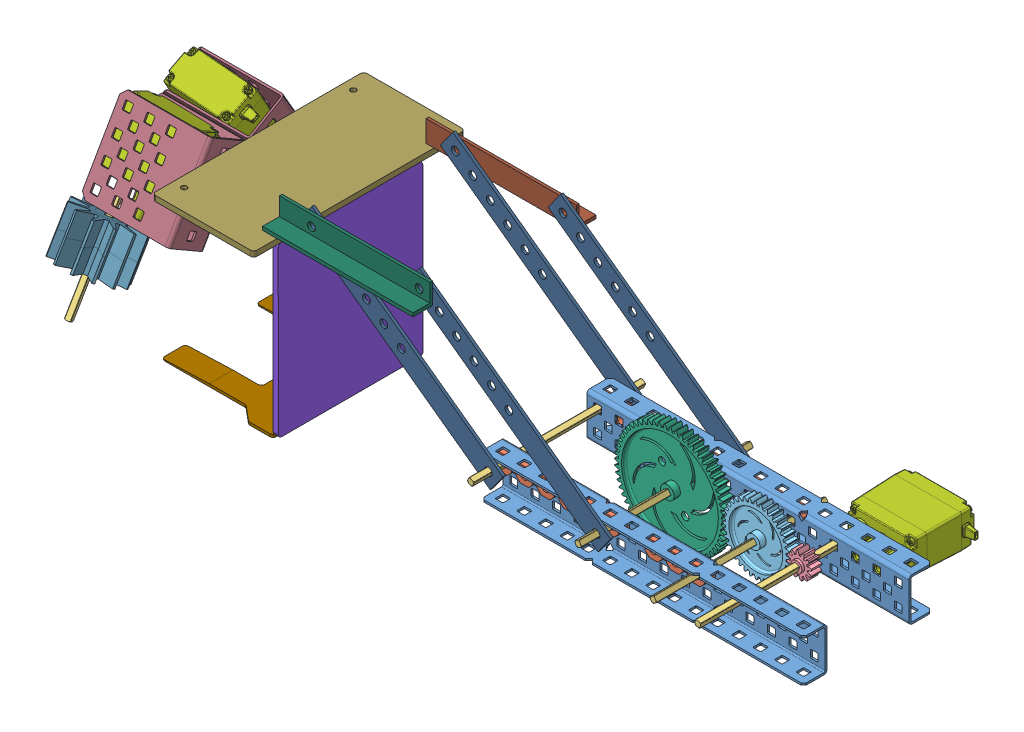
SolidWorks assembly LiftAssy-NoMates, configuration Default. Lengths in mm.
Overall size (436.18 185.84 157.73).
36 component instances, 15 part files, 3 mates.
Components (placement in the parent):
- VL-CHAN-121-15 RevA-1: VL-CHAN-121-15 RevA [Default] at (-291.0348 35.1994 12.7) x (1 0 0) z (0 -1 0) size (190.5 13.87 25.4)
- VL-CHAN-121-15 RevA-2: VL-CHAN-121-15 RevA [Default] at (-153.4652 35.1994 63.5) x (-1 0 0) z (0 -1 0) size (190.5 13.87 25.4)
- BEARING-FLAT-1: BEARING-FLAT [Default] at (-272.0848 31.6992 -76.2762) x (0 0 1) z (0 -1 0) size (7.04 35.56 10.16)
- BEARING-FLAT-2: BEARING-FLAT [Default] at (-233.9848 31.8008 -76.2762) x (0 0 1) z (0 -1 0) size (7.04 35.56 10.16)
- BEARING-FLAT-3: BEARING-FLAT [Default] at (-183.1848 57.2008 152.4762) x (0 0 -1) z (0 1 0) size (7.04 35.56 10.16)
- BEARING-FLAT-4: BEARING-FLAT [Default] at (-235.9152 57.2008 -76.2762) x (0 0 1) z (0 1 0) size (7.04 35.56 10.16)
- BEARING-FLAT-5: BEARING-FLAT [Default] at (-233.9848 57.2008 152.4762) x (0 0 -1) z (0 1 0) size (7.04 35.56 10.16)
- BEARING-FLAT-6: BEARING-FLAT [Default] at (-272.0848 57.2008 152.4762) x (0 0 -1) z (0 1 0) size (7.04 35.56 10.16)
- SHAFT-4000-1: SHAFT-4000 [Default] at (-311.2008 44.5008 38.1) x (0.41269 0.910872 0) z (0 0 1) size (4.18 4.18 101.81)
- SHAFT-4000-2: SHAFT-4000 [Default] at (-247.7008 44.5008 38.1) x (0.537594 -0.843204 0) z (0 0 1) size (4.18 4.18 101.81)
- SHAFT-4000-3: SHAFT-4000 [Default] at (-196.9008 44.5008 44.45) x (0.810991 0.585059 0) z (0 0 1) size (4.18 4.18 101.81)
- SHAFT-4000-4: SHAFT-4000 [Default] at (-171.4187 44.4677 43.6) x (0.963526 -0.267616 0) z (0 0 1) size (4.18 4.18 101.81)
- VEX-12-TOOTH-GEAR-1: VEX-12-TOOTH-GEAR [Default] at (-171.388 44.4851 31.3309) x (0.963526 -0.267616 0) z (0 0 1) size (14.8 14.8 9.53)
- VEX-36-TOOTH-GEAR-1: VEX-36-TOOTH-GEAR [Default] at (-196.9357 44.5064 31.3309) x (0.810991 0.585059 0) z (0 0 1) size (40.08 40.08 9.53)
- VEX-60-TOOTH-GEAR-1: VEX-60-TOOTH-GEAR [Default] at (-247.7353 44.5084 31.3309) x (0.537594 -0.843204 0) z (0 0 1) size (65.54 65.54 9.53)
- VEX-2WIRE-MOTOR-1: VEX-2WIRE-MOTOR [Default] at (-160.3202 44.45 -30.5) x (-1 0 0) z (0 0 -1) size (46.4 20 51.81)
- Pyramid Intake-1: Pyramid Intake [Default] at (-389.3852 43.5371 -4.7167) x (0 0 1) z (-0.989362 0.145478 0) size (150.3 140.72 320.47)
  - back-1: back [Default] at (51.2746 60.4405 44.4758) x (1 0 0) z (0 -0.146963 0.989142) size (85.5 99.5 3.17)
  - BottomForklift-1: BottomForklift [Default] at (51.2746 -40.016 32.7601) x (1 0 0) z (0 -0.146963 0.989142) size (85.5 1.59 73.7)
  - Circles 5.5in Inch Shaft Bar-1: Circles 5.5in Inch Shaft Bar [Default] at (81.5651 21.6246 -45.8337) x (0 0.885997 -0.463691) z (0 -0.463691 -0.885997) size (12.7 1.59 139.7)
  - Circles 5.5in Inch Shaft Bar-2: Circles 5.5in Inch Shaft Bar [Default] at (81.5651 30.9788 -108.7925) x (0 0.885997 -0.463691) z (0 -0.463691 -0.885997) size (12.7 1.59 139.7)
  - Circles 5.5in Inch Shaft Bar-3: Circles 5.5in Inch Shaft Bar [Default] at (1.9185 22.2168 -49.6344) x (0 0.885997 -0.463691) z (0 -0.463691 -0.885997) size (12.7 1.59 139.7)
  - Circles 5.5in Inch Shaft Bar-4: Circles 5.5in Inch Shaft Bar [Default] at (1.9185 31.571 -112.5933) x (0 0.885997 -0.463691) z (0 -0.463691 -0.885997) size (12.7 1.59 139.7)
  - Circles 3.5 inch Linkage-4: Circles 3.5 inch Linkage [Default] at (1.9185 61.0879 62.0444) x (0 0.989142 0.146963) z (0 -0.146963 0.989142) size (12.75 11.59 88.91)
  - top-2: top [Default] at (45.9604 60.4405 44.4758) x (1 0 0) z (0 -0.146963 0.989142) size (125 3.17 60)
  - VL-RACK-BRK RevA-1: VL-RACK-BRK RevA [Default] at (75.6784 37.9578 101.794) x (-0.866025 -0.494571 -0.073482) z (-0.5 0.856622 0.127274) size (24.56 52.4 50.8)
  - VL-RACK-BRK RevA-2: VL-RACK-BRK RevA [Default] at (27.9082 38.1401 101.8211) x (-0.866025 0.494571 0.073482) z (0.5 0.856622 0.127274) size (24.56 52.4 50.8)
  - VEX-2WIRE-MOTOR-1: VEX-2WIRE-MOTOR [Default] at (37.2345 49.19 137.8585) x (-0.036906 -0.095703 0.994726) z (0.523598 0.845979 0.100819) size (46.4 20 51.81)
  - VEX-2WIRE-MOTOR-2: VEX-2WIRE-MOTOR [Default] at (66.0042 45.7522 136.293) x (0.02622 -0.1019 0.994449) z (-0.478039 0.872396 0.101997) size (46.4 20 51.81)
  - SHAFT-4000-1: SHAFT-4000 [Default] at (87.1245 6.543 142.8927) x (0.260216 0.029754 0.965092) z (-0.478039 0.872396 0.101997) size (4.18 4.18 101.81)
  - SHAFT-4000-2: SHAFT-4000 [Default] at (13.8193 10.8964 144.5121) x (0.829997 -0.479812 -0.284404) z (0.523598 0.845979 0.100819) size (4.18 4.18 101.81)
  - INTAKE-ROLLER-1: INTAKE-ROLLER [Default] at (-2.7854 -15.9478 141.2978) x (0.248526 -0.038475 -0.967861) z (0.523598 0.845979 0.100819) size (38.1 38.1 12.7)
  - INTAKE-ROLLER-2: INTAKE-ROLLER [Default] at (3.8643 -5.2039 142.5782) x (-0.192226 0.232592 -0.953389) z (0.523598 0.845979 0.100819) size (38.1 38.1 12.7)
  - INTAKE-ROLLER-3: INTAKE-ROLLER [Default] at (91.181 -0.8787 142.0407) x (0.260216 0.029754 0.965092) z (0.478039 -0.872396 -0.101997) size (38.1 38.1 12.7)
  - INTAKE-ROLLER-4: INTAKE-ROLLER [Default] at (97.2521 -11.9581 140.7453) x (-0.596407 -0.407651 0.691462) z (0.478039 -0.872396 -0.101997) size (38.1 38.1 12.7)
  - Circles 3.5 inch Linkage-o-1: Circles 3.5 inch Linkage-o [Default] at (84.7401 60.4957 65.8452) x (0 0.989142 0.146963) z (0 -0.146963 0.989142) size (12.72 11.59 88.94)
Mates (geometry in assembly coordinates):
- Width1: width: plane of SHAFT-4000-1 through (-309.0997 45.2917 88.9) normal (0.41269 0.910872 0); plane of SHAFT-4000-1 through (-310.4099 42.3996 88.9) normal (-0.41269 -0.910872 0); cylinder of Pyramid Intake-1/Circles 5.5in Inch Shaft Bar-1 through (-311.2008 44.5008 78.4359) axis (0 0 -1) radius 2.31
- Width2: width: plane of SHAFT-4000-1 through (-313.302 43.7099 88.9) normal (-0.910872 0.41269 0); plane of SHAFT-4000-1 through (-310.4099 42.3996 88.9) normal (0.910872 -0.41269 0); cylinder of Pyramid Intake-1/Circles 5.5in Inch Shaft Bar-1 through (-311.2008 44.5008 78.4359) axis (0 0 -1) radius 2.31
- Width3: width: plane of SHAFT-4000-2 through (-249.8928 44.986 88.9) normal (-0.537594 0.843204 0); plane of SHAFT-4000-2 through (-248.186 42.3088 88.9) normal (0.537594 -0.843204 0); cylinder of Pyramid Intake-1/Circles 5.5in Inch Shaft Bar-2 through (-247.5509 44.5964 78.4359) axis (0 0 -1) radius 2.31
